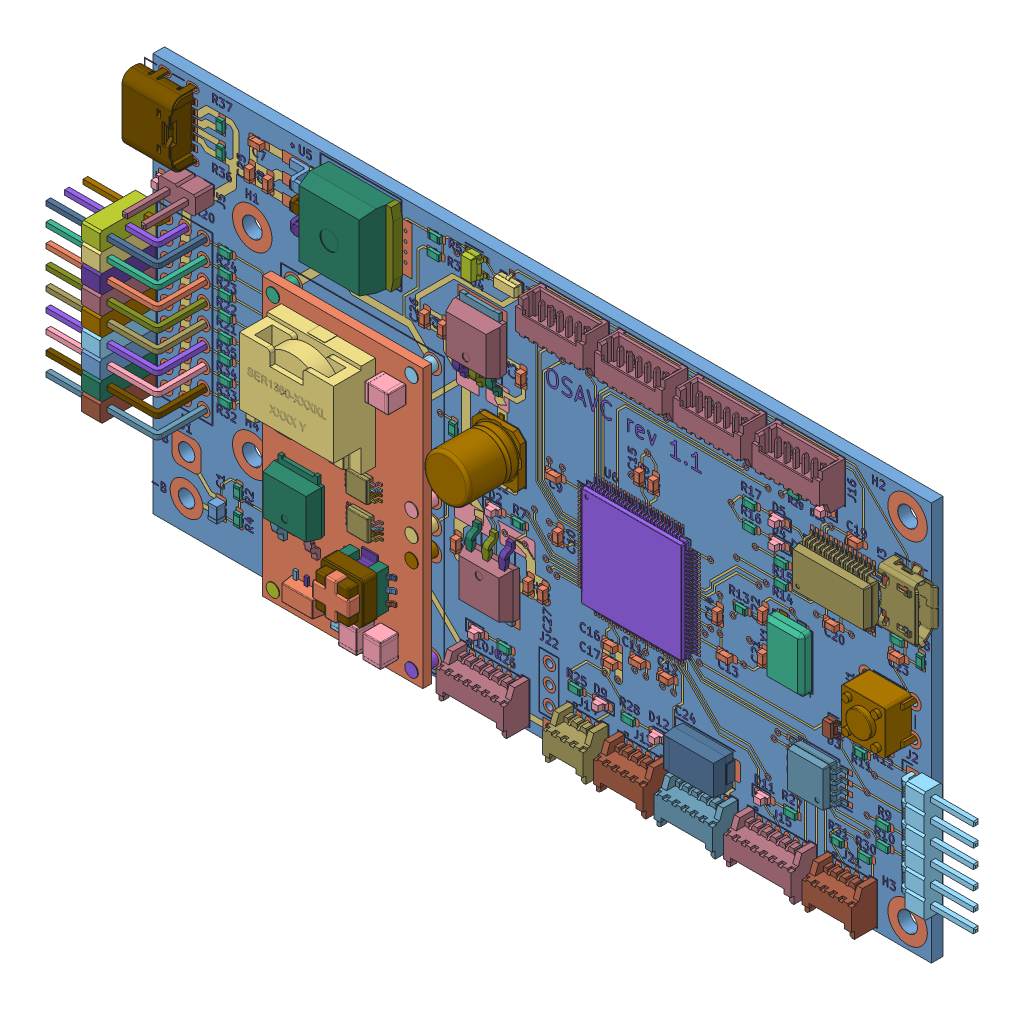
SolidWorks assembly OSAVC_rev1.1, configuration Default. Lengths in mm.
Overall size (122.32 54.61 12.06).
260 component instances, 123 part files, 0 mates.
Components (placement in the parent):
- OSAVC_rev1.1.step-1: OSAVC_rev1.1.step [Default] at origin size (122.32 54.61 12.06)
  - Local_CS_6c55.step-1: Local_CS_6c55.step [Default] at origin
  - Board_Geoms_6c55.step-1: Board_Geoms_6c55.step [Default] at origin size (107.79 54.61 2.3)
    - Pcb_6c55.step-1: Pcb_6c55.step [Default] at (-86.36 81.28 0) size (106.68 54.61 1.6)
    - PCB_Sketch_6c55.step-1: PCB_Sketch_6c55.step [Default] at origin
    - topPads_6c55_cut.step-1: topPads_6c55_cut.step [Default] at (0 0 0.02) size (105.36 53.51 0.01)
    - topTracks_6c55.step-1: topTracks_6c55.step [Default] at (-86.36 81.28 0.01) size (104.4 52.61 0.07)
    - topZones_6c55.step-1: topZones_6c55.step [Default] at (-86.36 81.28 0.01) size (10.98 18.86 0.02)
    - botPads_6c55.step-1: botPads_6c55.step [Default] at (-86.36 81.28 -1.62) size (105.31 53.51 0.01)
    - botTracks_6c55.step-1: botTracks_6c55.step [Default] at (-86.36 81.28 -1.61) size (93.18 51.32 0.63)
    - botSilks_69b0.step-1: botSilks_69b0.step [Default] at (-86.36 81.28 -1.67) size (102.66 52.04 0.03)
    - topSilks_6464.step-1: topSilks_6464.step [Default] at (-86.36 81.28 0.07) size (107.59 54.1 0.61)
  - Step_Models_6c55.step-1: Step_Models_6c55.step [Default] at origin size (122.32 53.45 12.06)
    - Top_6c55.step-1: Top_6c55.step [Default] at origin size (122.32 53.45 12.06)
      - C2_C_Elec_63x079_00006184c965.step-1: C2_C_Elec_63x079_00006184c965.step [Default] at (47.89 -22.72 0) x (0 -1 0) z (0 0 1) size (8.61 8.6 7.7)
        - C_Elec_63x77.step-1: C_Elec_63x77.step [Default] at origin size (8.61 8.6 7.7)
        - C_Elec_63x078.step-1: C_Elec_63x078.step [Default] at origin size (0.02 0.02 0.01)
      - J4_PinHeader_3x09_P2.54mm_Horizontal036_00006184cc7d.step-1: J4_PinHeader_3x09_P2.54mm_Horizontal036_00006184cc7d.step [Default] at (6.985 -38.735 0) x (-1 0 0) z (0 0 1) size (15.44 22.86 10.62)
        - PinHeader_3x09_P2.54mm_Horizontal.step-1: PinHeader_3x09_P2.54mm_Horizontal.step [Default] at origin size (2.54 2.54 7.62)
        - PinHeader_3x09_P2.54mm_Horizontal001.step-1: PinHeader_3x09_P2.54mm_Horizontal001.step [Default] at origin size (12.9 0.64 7.13)
        - PinHeader_3x09_P2.54mm_Horizontal002.step-1: PinHeader_3x09_P2.54mm_Horizontal002.step [Default] at origin size (10.36 0.64 4.59)
        - PinHeader_3x09_P2.54mm_Horizontal003.step-1: PinHeader_3x09_P2.54mm_Horizontal003.step [Default] at origin size (15.44 0.64 9.67)
        - PinHeader_3x09_P2.54mm_Horizontal004.step-1: PinHeader_3x09_P2.54mm_Horizontal004.step [Default] at origin size (2.54 2.54 7.62)
        - PinHeader_3x09_P2.54mm_Horizontal005.step-1: PinHeader_3x09_P2.54mm_Horizontal005.step [Default] at origin size (12.9 0.64 7.13)
        - PinHeader_3x09_P2.54mm_Horizontal006.step-1: PinHeader_3x09_P2.54mm_Horizontal006.step [Default] at origin size (10.36 0.64 4.59)
        - PinHeader_3x09_P2.54mm_Horizontal007.step-1: PinHeader_3x09_P2.54mm_Horizontal007.step [Default] at origin size (15.44 0.64 9.67)
        - PinHeader_3x09_P2.54mm_Horizontal008.step-1: PinHeader_3x09_P2.54mm_Horizontal008.step [Default] at origin size (2.54 2.54 7.62)
        - PinHeader_3x09_P2.54mm_Horizontal009.step-1: PinHeader_3x09_P2.54mm_Horizontal009.step [Default] at origin size (12.9 0.64 7.13)
        - PinHeader_3x09_P2.54mm_Horizontal010.step-1: PinHeader_3x09_P2.54mm_Horizontal010.step [Default] at origin size (10.36 0.64 4.59)
        - PinHeader_3x09_P2.54mm_Horizontal011.step-1: PinHeader_3x09_P2.54mm_Horizontal011.step [Default] at origin size (15.44 0.64 9.67)
        - PinHeader_3x09_P2.54mm_Horizontal012.step-1: PinHeader_3x09_P2.54mm_Horizontal012.step [Default] at origin size (2.54 2.54 7.62)
        - PinHeader_3x09_P2.54mm_Horizontal013.step-1: PinHeader_3x09_P2.54mm_Horizontal013.step [Default] at origin size (12.9 0.64 7.13)
        - PinHeader_3x09_P2.54mm_Horizontal014.step-1: PinHeader_3x09_P2.54mm_Horizontal014.step [Default] at origin size (10.36 0.64 4.59)
        - PinHeader_3x09_P2.54mm_Horizontal015.step-1: PinHeader_3x09_P2.54mm_Horizontal015.step [Default] at origin size (15.44 0.64 9.67)
        - PinHeader_3x09_P2.54mm_Horizontal016.step-1: PinHeader_3x09_P2.54mm_Horizontal016.step [Default] at origin size (2.54 2.54 7.62)
        - PinHeader_3x09_P2.54mm_Horizontal017.step-1: PinHeader_3x09_P2.54mm_Horizontal017.step [Default] at origin size (12.9 0.64 7.13)
        - PinHeader_3x09_P2.54mm_Horizontal018.step-1: PinHeader_3x09_P2.54mm_Horizontal018.step [Default] at origin size (10.36 0.64 4.59)
        - PinHeader_3x09_P2.54mm_Horizontal019.step-1: PinHeader_3x09_P2.54mm_Horizontal019.step [Default] at origin size (15.44 0.64 9.67)
        - PinHeader_3x09_P2.54mm_Horizontal020.step-1: PinHeader_3x09_P2.54mm_Horizontal020.step [Default] at origin size (2.54 2.54 7.62)
        - PinHeader_3x09_P2.54mm_Horizontal021.step-1: PinHeader_3x09_P2.54mm_Horizontal021.step [Default] at origin size (12.9 0.64 7.13)
        - PinHeader_3x09_P2.54mm_Horizontal022.step-1: PinHeader_3x09_P2.54mm_Horizontal022.step [Default] at origin size (10.36 0.64 4.59)
        - PinHeader_3x09_P2.54mm_Horizontal023.step-1: PinHeader_3x09_P2.54mm_Horizontal023.step [Default] at origin size (15.44 0.64 9.67)
        - PinHeader_3x09_P2.54mm_Horizontal024.step-1: PinHeader_3x09_P2.54mm_Horizontal024.step [Default] at origin size (2.54 2.54 7.62)
        - PinHeader_3x09_P2.54mm_Horizontal025.step-1: PinHeader_3x09_P2.54mm_Horizontal025.step [Default] at origin size (12.9 0.64 7.13)
        - PinHeader_3x09_P2.54mm_Horizontal026.step-1: PinHeader_3x09_P2.54mm_Horizontal026.step [Default] at origin size (10.36 0.64 4.59)
        - PinHeader_3x09_P2.54mm_Horizontal027.step-1: PinHeader_3x09_P2.54mm_Horizontal027.step [Default] at origin size (15.44 0.64 9.67)
        - PinHeader_3x09_P2.54mm_Horizontal028.step-1: PinHeader_3x09_P2.54mm_Horizontal028.step [Default] at origin size (2.54 2.54 7.62)
        - PinHeader_3x09_P2.54mm_Horizontal029.step-1: PinHeader_3x09_P2.54mm_Horizontal029.step [Default] at origin size (12.9 0.64 7.13)
        - PinHeader_3x09_P2.54mm_Horizontal030.step-1: PinHeader_3x09_P2.54mm_Horizontal030.step [Default] at origin size (10.36 0.64 4.59)
        - PinHeader_3x09_P2.54mm_Horizontal031.step-1: PinHeader_3x09_P2.54mm_Horizontal031.step [Default] at origin size (15.44 0.64 9.67)
        - PinHeader_3x09_P2.54mm_Horizontal032.step-1: PinHeader_3x09_P2.54mm_Horizontal032.step [Default] at origin size (2.54 2.54 7.62)
        - PinHeader_3x09_P2.54mm_Horizontal033.step-1: PinHeader_3x09_P2.54mm_Horizontal033.step [Default] at origin size (12.9 0.64 7.13)
        - PinHeader_3x09_P2.54mm_Horizontal034.step-1: PinHeader_3x09_P2.54mm_Horizontal034.step [Default] at origin size (10.36 0.64 4.59)
        - PinHeader_3x09_P2.54mm_Horizontal035.step-1: PinHeader_3x09_P2.54mm_Horizontal035.step [Default] at origin size (15.44 0.64 9.67)
      - J13_Picoblade_horizontal_4p_00006184cca8.step-1: J13_Picoblade_horizontal_4p_00006184cca8.step [Default] at (65.405 -49.53 0) x (1 0 0) z (0 -1 0) size (6.75 5.8 5.5)
        - 530480410.step-1: 530480410.step [Default] at (1.875 1.9 3.475) x (-1 0 0) z (0 1 0) size (6.75 5.5 5.8)
      - J14_Picoblade_horizontal_3p_00006184ccd2.step-1: J14_Picoblade_horizontal_3p_00006184ccd2.step [Default] at (58.42 -49.53 0) x (1 0 0) z (0 -1 0) size (5.5 5.8 5.5)
        - 530480310.step-1: 530480310.step [Default] at (1.25 1.9 3.475) x (-1 0 0) z (0 1 0) size (5.5 5.5 5.8)
      - J15_Picoblade_horizontal_6p_00006184ccff.step-1: J15_Picoblade_horizontal_6p_00006184ccff.step [Default] at (83.185 -49.53 0) x (1 0 0) z (0 -1 0) size (9.25 5.8 5.5)
        - 530480610.step-1: 530480610.step [Default] at (3.125 1.9 3.475) x (-1 0 0) z (0 1 0) size (9.25 5.5 5.8)
      - J15_Picoblade_horizontal_6p_00006184ccff.step-2: J15_Picoblade_horizontal_6p_00006184ccff.step [Default] at (93.345 -5.08 0) x (-1 0 0) z (0 1 0) size (9.25 5.8 5.5)
        - 530480610.step-1: 530480610.step [Default] at (3.125 1.9 3.475) x (-1 0 0) z (0 1 0) size (9.25 5.5 5.8)
      - J15_Picoblade_horizontal_6p_00006184ccff.step-3: J15_Picoblade_horizontal_6p_00006184ccff.step [Default] at (82.55 -5.08 0) x (-1 0 0) z (0 1 0) size (9.25 5.8 5.5)
        - 530480610.step-1: 530480610.step [Default] at (3.125 1.9 3.475) x (-1 0 0) z (0 1 0) size (9.25 5.5 5.8)
      - J15_Picoblade_horizontal_6p_00006184ccff.step-4: J15_Picoblade_horizontal_6p_00006184ccff.step [Default] at (71.755 -5.08 0) x (-1 0 0) z (0 1 0) size (9.25 5.8 5.5)
        - 530480610.step-1: 530480610.step [Default] at (3.125 1.9 3.475) x (-1 0 0) z (0 1 0) size (9.25 5.5 5.8)
      - J20_Picoblade_horizontal_5p_00006184cddf.step-1: J20_Picoblade_horizontal_5p_00006184cddf.step [Default] at (73.66 -49.53 0) x (1 0 0) z (0 -1 0) size (8 5.8 5.5)
        - 530480510.step-1: 530480510.step [Default] at (2.5 1.9 3.475) x (-1 0 0) z (0 1 0) size (8 5.5 5.8)
      - J13_Picoblade_horizontal_4p_00006184cca8.step-2: J13_Picoblade_horizontal_4p_00006184cca8.step [Default] at (93.98 -49.53 0) x (1 0 0) z (0 -1 0) size (6.75 5.8 5.5)
        - 530480410.step-1: 530480410.step [Default] at (1.875 1.9 3.475) x (-1 0 0) z (0 1 0) size (6.75 5.5 5.8)
      - U5_CQ assembly_00006184d1ab.step-1: U5_CQ assembly_00006184d1ab.step [Default] at (28.575 -5.715 0) size (15 10 4.42)
        - a52d3816-9c39-11ed-93f0-dde97e994e83.step-1: a52d3816-9c39-11ed-93f0-dde97e994e83.step [Default] at origin size (15 10 4.42)
          - a52d3817-9c39-11ed-93f0-dde97e994e83.step-1: a52d3817-9c39-11ed-93f0-dde97e994e83.step [Default] at origin size (9.25 10 4.4)
            - a52d3817-9c39-11ed-93f0-dde97e994e83_part.step-1: a52d3817-9c39-11ed-93f0-dde97e994e83_part.step [Default] at origin size (9.25 10 4.4)
          - a52d3818-9c39-11ed-93f0-dde97e994e83.step-1: a52d3818-9c39-11ed-93f0-dde97e994e83.step [Default] at origin size (7.55 10 1.27)
            - a52d3818-9c39-11ed-93f0-dde97e994e83_part.step-1: a52d3818-9c39-11ed-93f0-dde97e994e83_part.step [Default] at origin size (7.55 10 1.27)
          - a52d3819-9c39-11ed-93f0-dde97e994e83.step-1: a52d3819-9c39-11ed-93f0-dde97e994e83.step [Default] at origin size (4.95 6.32 2.95)
            - a52d3819-9c39-11ed-93f0-dde97e994e83_part003.step-1: a52d3819-9c39-11ed-93f0-dde97e994e83_part003.step [Default] at origin size (4.95 6.32 2.95)
              - a52d3819-9c39-11ed-93f0-dde97e994e83_part.step-1: a52d3819-9c39-11ed-93f0-dde97e994e83_part.step [Default] at origin size (4.95 1.24 2.95)
              - a52d3819-9c39-11ed-93f0-dde97e994e83_part001.step-1: a52d3819-9c39-11ed-93f0-dde97e994e83_part001.step [Default] at origin size (4.95 1.24 2.95)
              - a52d3819-9c39-11ed-93f0-dde97e994e83_part002.step-1: a52d3819-9c39-11ed-93f0-dde97e994e83_part002.step [Default] at origin size (4.95 1.24 2.95)
      - J15_Picoblade_horizontal_6p_00006184ccff.step-5: J15_Picoblade_horizontal_6p_00006184ccff.step [Default] at (43.815 -49.53 0) x (1 0 0) z (0 -1 0) size (9.25 5.8 5.5)
        - 530480610.step-1: 530480610.step [Default] at (3.125 1.9 3.475) x (-1 0 0) z (0 1 0) size (9.25 5.5 5.8)
      - U1_PTN78020W_EUK-7_00006189aa32.step-1: U1_PTN78020W_EUK-7_00006189aa32.step [Default] at (19.304 -52.578 0) x (1 0 0) z (0 -1 0) size (22 12 38)
        - Board^Voltage_regulator.STEP008.step-1: Board^Voltage_regulator.STEP008.step [Default] at origin size (22 6.34 38)
          - Board^Voltage_regulator.STEP.step-1: Board^Voltage_regulator.STEP.step [Default] at origin size (22 1.2 38)
          - Board^Voltage_regulator.STEP001.step-1: Board^Voltage_regulator.STEP001.step [Default] at origin size (1.75 6.34 1.75)
          - Board^Voltage_regulator.STEP002.step-1: Board^Voltage_regulator.STEP002.step [Default] at origin size (1.75 6.34 1.75)
          - Board^Voltage_regulator.STEP003.step-1: Board^Voltage_regulator.STEP003.step [Default] at origin size (1.75 6.34 1.75)
          - Board^Voltage_regulator.STEP004.step-1: Board^Voltage_regulator.STEP004.step [Default] at origin size (1.75 6.34 1.75)
          - Board^Voltage_regulator.STEP005.step-1: Board^Voltage_regulator.STEP005.step [Default] at origin size (1.75 6.34 1.75)
          - Board^Voltage_regulator.STEP006.step-1: Board^Voltage_regulator.STEP006.step [Default] at origin size (1.75 6.34 1.75)
          - Board^Voltage_regulator.STEP007.step-1: Board^Voltage_regulator.STEP007.step [Default] at origin size (1.75 6.34 1.75)
        - SMTCurrentSenseTransformer.STEP011.step-1: SMTCurrentSenseTransformer.STEP011.step [Default] at origin size (7.12 5.58 6.13)
          - SMTCurrentSenseTransformer.STEP.step-1: SMTCurrentSenseTransformer.STEP.step [Default] at (13.366 2.8 -8.2501) size (0.93 0.55 0.52)
          - SMTCurrentSenseTransformer.STEP001.step-1: SMTCurrentSenseTransformer.STEP001.step [Default] at (13.366 2.8 -8.2501) size (0.93 0.55 0.52)
          - SMTCurrentSenseTransformer.STEP002.step-1: SMTCurrentSenseTransformer.STEP002.step [Default] at (13.366 2.8 -8.2501) size (0.93 0.55 0.52)
          - SMTCurrentSenseTransformer.STEP003.step-1: SMTCurrentSenseTransformer.STEP003.step [Default] at (13.366 2.8 -8.2501) size (0.93 0.55 0.52)
          - SMTCurrentSenseTransformer.STEP004.step-1: SMTCurrentSenseTransformer.STEP004.step [Default] at (13.366 2.8 -8.2501) size (0.93 0.55 0.52)
          - SMTCurrentSenseTransformer.STEP005.step-1: SMTCurrentSenseTransformer.STEP005.step [Default] at (13.366 2.8 -8.2501) size (5.27 1.76 5.27)
          - SMTCurrentSenseTransformer.STEP006.step-1: SMTCurrentSenseTransformer.STEP006.step [Default] at (13.366 2.8 -8.2501) size (2.16 1.97 1.51)
          - SMTCurrentSenseTransformer.STEP007.step-1: SMTCurrentSenseTransformer.STEP007.step [Default] at (13.366 2.8 -8.2501) size (2.16 1.97 1.51)
          - SMTCurrentSenseTransformer.STEP008.step-1: SMTCurrentSenseTransformer.STEP008.step [Default] at (13.366 2.8 -8.2501) size (5.7 3.39 5.7)
          - SMTCurrentSenseTransformer.STEP009.step-1: SMTCurrentSenseTransformer.STEP009.step [Default] at (13.366 2.8 -8.2501) size (0.93 0.55 0.52)
          - SMTCurrentSenseTransformer.STEP010.step-1: SMTCurrentSenseTransformer.STEP010.step [Default] at (13.366 2.8 -8.2501) size (5.02 1.55 5.02)
        - MSOP-8.STEP010.step-1: MSOP-8.STEP010.step [Default] at origin size (4.9 1.1 3)
          - MSOP-8.STEP.step-1: MSOP-8.STEP.step [Default] at (12.6175 3.1325 -15.6358) x (0 -1 0) z (-1 0 0) size (0.67 0.44 1.43)
          - MSOP-8.STEP001.step-1: MSOP-8.STEP001.step [Default] at (12.6175 3.1325 -15.6358) x (0 -1 0) z (-1 0 0) size (0.67 0.44 1.43)
          - MSOP-8.STEP002.step-1: MSOP-8.STEP002.step [Default] at (12.6175 3.1325 -15.6358) x (0 -1 0) z (-1 0 0) size (0.67 0.44 1.43)
          - MSOP-8.STEP003.step-1: MSOP-8.STEP003.step [Default] at (12.6175 3.1325 -15.6358) x (0 -1 0) z (-1 0 0) size (0.67 0.44 1.43)
          - MSOP-8.STEP004.step-1: MSOP-8.STEP004.step [Default] at (12.6175 3.1325 -15.6358) x (0 -1 0) z (-1 0 0) size (0.67 0.44 1.43)
          - MSOP-8.STEP005.step-1: MSOP-8.STEP005.step [Default] at (12.6175 3.1325 -15.6358) x (0 -1 0) z (-1 0 0) size (0.15 2.39 1.73)
          - MSOP-8.STEP006.step-1: MSOP-8.STEP006.step [Default] at (12.6175 3.1325 -15.6358) x (0 -1 0) z (-1 0 0) size (0.67 0.44 1.43)
          - MSOP-8.STEP007.step-1: MSOP-8.STEP007.step [Default] at (12.6175 3.1325 -15.6358) x (0 -1 0) z (-1 0 0) size (0.67 0.44 1.43)
          - MSOP-8.STEP008.step-1: MSOP-8.STEP008.step [Default] at (12.6175 3.1325 -15.6358) x (0 -1 0) z (-1 0 0) size (0.67 0.44 1.43)
          - MSOP-8.STEP009.step-1: MSOP-8.STEP009.step [Default] at (12.6175 3.1325 -15.6358) x (0 -1 0) z (-1 0 0) size (0.94 3 3.01)
        - MSOP-8.STEP021.step-1: MSOP-8.STEP021.step [Default] at origin size (4.9 1.1 3)
          - MSOP-8.STEP.step-1: MSOP-8.STEP.step [Default] at (12.5011 3.1325 -20.1358) x (0 -1 0) z (-1 0 0) size (0.67 0.44 1.43)
          - MSOP-8.STEP001.step-1: MSOP-8.STEP001.step [Default] at (12.5011 3.1325 -20.1358) x (0 -1 0) z (-1 0 0) size (0.67 0.44 1.43)
          - MSOP-8.STEP002.step-1: MSOP-8.STEP002.step [Default] at (12.5011 3.1325 -20.1358) x (0 -1 0) z (-1 0 0) size (0.67 0.44 1.43)
          - MSOP-8.STEP003.step-1: MSOP-8.STEP003.step [Default] at (12.5011 3.1325 -20.1358) x (0 -1 0) z (-1 0 0) size (0.67 0.44 1.43)
          - MSOP-8.STEP004.step-1: MSOP-8.STEP004.step [Default] at (12.5011 3.1325 -20.1358) x (0 -1 0) z (-1 0 0) size (0.67 0.44 1.43)
          - MSOP-8.STEP005.step-1: MSOP-8.STEP005.step [Default] at (12.5011 3.1325 -20.1358) x (0 -1 0) z (-1 0 0) size (0.15 2.39 1.73)
          - MSOP-8.STEP006.step-1: MSOP-8.STEP006.step [Default] at (12.5011 3.1325 -20.1358) x (0 -1 0) z (-1 0 0) size (0.67 0.44 1.43)
          - MSOP-8.STEP007.step-1: MSOP-8.STEP007.step [Default] at (12.5011 3.1325 -20.1358) x (0 -1 0) z (-1 0 0) size (0.67 0.44 1.43)
          - MSOP-8.STEP008.step-1: MSOP-8.STEP008.step [Default] at (12.5011 3.1325 -20.1358) x (0 -1 0) z (-1 0 0) size (0.67 0.44 1.43)
          - MSOP-8.STEP009.step-1: MSOP-8.STEP009.step [Default] at (12.5011 3.1325 -20.1358) x (0 -1 0) z (-1 0 0) size (0.94 3 3.01)
        - DPAK.STEP004.step-1: DPAK.STEP004.step [Default] at origin size (6.5 2.3 9.95)
          - DPAK.STEP.step-1: DPAK.STEP.step [Default] at (3.8382 3.3 -12.8868) size (1 1.4 3.06)
          - DPAK.STEP001.step-1: DPAK.STEP001.step [Default] at (3.8382 3.3 -12.8868) size (1 1.4 3.06)
          - DPAK.STEP002.step-1: DPAK.STEP002.step [Default] at (3.8382 3.3 -12.8868) size (6.5 2.3 7.05)
          - DPAK.STEP003.step-1: DPAK.STEP003.step [Default] at (3.8382 3.3 -12.8868) size (0.9 0.5 0.8)
        - SOT89.STEP004.step-1: SOT89.STEP004.step [Default] at origin size (4.5 1.5 4.13)
          - SOT89.STEP.step-1: SOT89.STEP.step [Default] at (4.7525 3.13 -2) x (-1 0 0) z (0 0 1) size (1.6 0.33 4.13)
          - SOT89.STEP001.step-1: SOT89.STEP001.step [Default] at (4.7525 3.13 -2) x (-1 0 0) z (0 0 1) size (0.47 0.33 1.48)
          - SOT89.STEP002.step-1: SOT89.STEP002.step [Default] at (4.7525 3.13 -2) x (-1 0 0) z (0 0 1) size (0.47 0.33 1.48)
          - SOT89.STEP003.step-1: SOT89.STEP003.step [Default] at (4.7525 3.13 -2) x (-1 0 0) z (0 0 1) size (4.5 1.5 2.5)
        - Coilcraft-SER1360.STEP.step-1: Coilcraft-SER1360.STEP.step [Default] at (7.55 2.8 -28.05) x (0 0 1) z (-1 0 0) size (13 5.81 12.9)
        - SMD_Capacitor_1210_1210.STEP.step-1: SMD_Capacitor_1210_1210.STEP.step [Default] at (15.94 4.04 -1.9) x (0 0 1) z (-1 0 0) size (3.2 2.5 2.5)
        - SMD_Capacitor_1210_1210.STEP.step-2: SMD_Capacitor_1210_1210.STEP.step [Default] at (12.64 4.04 -1.9) x (0 0 1) z (-1 0 0) size (3.2 2.5 2.5)
        - SMD_Capacitor_1210_1210.STEP.step-3: SMD_Capacitor_1210_1210.STEP.step [Default] at (16.6 4.04 -32.26) size (3.2 2.5 2.5)
        - SMD_Capacitor_0805_0805.STEP.step-1: SMD_Capacitor_0805_0805.STEP.step [Default] at (9.715 3.44 -1.625) x (0 0 -1) z (-1 0 0) size (2 1.3 1.25)
      - J15_Picoblade_horizontal_6p_00006184ccff.step-6: J15_Picoblade_horizontal_6p_00006184ccff.step [Default] at (60.96 -5.08 0) x (-1 0 0) z (0 1 0) size (9.25 5.8 5.5)
        - 530480610.step-1: 530480610.step [Default] at (3.125 1.9 3.475) x (-1 0 0) z (0 1 0) size (9.25 5.5 5.8)
      - Y1_SMD_crystal005_0000618b2749.step-1: Y1_SMD_crystal005_0000618b2749.step [Default] at (87.757 -27.051 0) x (0 1 0) z (0 0 1) size (8.22 5.2 1.5)
        - SMD_crystal.step-1: SMD_crystal.step [Default] at origin size (7.5 5.2 1.4)
        - SMD_crystal001.step-1: SMD_crystal001.step [Default] at origin size (1.92 1.12 0.1)
        - SMD_crystal002.step-1: SMD_crystal002.step [Default] at origin size (1.92 1.12 0.1)
        - SMD_crystal003.step-1: SMD_crystal003.step [Default] at origin size (1.92 1.12 0.1)
        - SMD_crystal004.step-1: SMD_crystal004.step [Default] at origin size (1.92 1.12 0.1)
      - J3_10118193003_0000618b348a.step-1: J3_10118193003_0000618b348a.step [Default] at (104.805 -12.065 0) x (0 1 0) z (1 0 0) size (7.87 3.61 5.71)
        - 10118193002.step-1: 10118193002.step [Default] at origin size (7.87 3.61 5.71)
          - 10118193.step-1: 10118193.step [Default] at (-0.19 0.055 -0.3676) size (6.89 2.35 4.32)
          - 10118193001.step-1: 10118193001.step [Default] at (-0.19 0.055 -0.3676) size (7.87 3.61 5.67)
      - U3_CQ assembly_0000618ecb8d.step-1: U3_CQ assembly_0000618ecb8d.step [Default] at (46.99 -38.8526 0) x (0 -1 0) z (0 0 1) size (9.9 6.5 2.32)
        - 98f8d7e0-9c39-11ed-93f0-dde97e994e83.step-1: 98f8d7e0-9c39-11ed-93f0-dde97e994e83.step [Default] at origin size (9.9 6.5 2.32)
          - 98f8d7e1-9c39-11ed-93f0-dde97e994e83.step-1: 98f8d7e1-9c39-11ed-93f0-dde97e994e83.step [Default] at origin size (6.22 6.5 2.3)
            - 98f8d7e1-9c39-11ed-93f0-dde97e994e83_part.step-1: 98f8d7e1-9c39-11ed-93f0-dde97e994e83_part.step [Default] at origin size (6.22 6.5 2.3)
          - 98f8d7e2-9c39-11ed-93f0-dde97e994e83.step-1: 98f8d7e2-9c39-11ed-93f0-dde97e994e83.step [Default] at origin size (5.24 5.4 0.5)
            - 98f8d7e2-9c39-11ed-93f0-dde97e994e83_part.step-1: 98f8d7e2-9c39-11ed-93f0-dde97e994e83_part.step [Default] at origin size (5.24 5.4 0.5)
          - 98f8d7e3-9c39-11ed-93f0-dde97e994e83.step-1: 98f8d7e3-9c39-11ed-93f0-dde97e994e83.step [Default] at origin size (3.55 5.55 1.44)
            - 98f8d7e3-9c39-11ed-93f0-dde97e994e83_part003.step-1: 98f8d7e3-9c39-11ed-93f0-dde97e994e83_part003.step [Default] at origin size (3.55 5.55 1.44)
              - 98f8d7e3-9c39-11ed-93f0-dde97e994e83_part.step-1: 98f8d7e3-9c39-11ed-93f0-dde97e994e83_part.step [Default] at origin size (3.55 0.99 1.44)
              - 98f8d7e3-9c39-11ed-93f0-dde97e994e83_part001.step-1: 98f8d7e3-9c39-11ed-93f0-dde97e994e83_part001.step [Default] at origin size (3.55 0.99 1.44)
              - 98f8d7e3-9c39-11ed-93f0-dde97e994e83_part002.step-1: 98f8d7e3-9c39-11ed-93f0-dde97e994e83_part002.step [Default] at origin size (3.55 0.99 1.44)
      - U3_CQ assembly_0000618ecb8d.step-2: U3_CQ assembly_0000618ecb8d.step [Default] at (45.212 -10.8044 0) x (0 1 0) z (0 0 1) size (9.9 6.5 2.32)
        - 98f8d7e0-9c39-11ed-93f0-dde97e994e83.step-1: 98f8d7e0-9c39-11ed-93f0-dde97e994e83.step [Default] at origin size (9.9 6.5 2.32)
          - 98f8d7e1-9c39-11ed-93f0-dde97e994e83.step-1: 98f8d7e1-9c39-11ed-93f0-dde97e994e83.step [Default] at origin size (6.22 6.5 2.3)
            - 98f8d7e1-9c39-11ed-93f0-dde97e994e83_part.step-1: 98f8d7e1-9c39-11ed-93f0-dde97e994e83_part.step [Default] at origin size (6.22 6.5 2.3)
          - 98f8d7e2-9c39-11ed-93f0-dde97e994e83.step-1: 98f8d7e2-9c39-11ed-93f0-dde97e994e83.step [Default] at origin size (5.24 5.4 0.5)
            - 98f8d7e2-9c39-11ed-93f0-dde97e994e83_part.step-1: 98f8d7e2-9c39-11ed-93f0-dde97e994e83_part.step [Default] at origin size (5.24 5.4 0.5)
          - 98f8d7e3-9c39-11ed-93f0-dde97e994e83.step-1: 98f8d7e3-9c39-11ed-93f0-dde97e994e83.step [Default] at origin size (3.55 5.55 1.44)
            - 98f8d7e3-9c39-11ed-93f0-dde97e994e83_part003.step-1: 98f8d7e3-9c39-11ed-93f0-dde97e994e83_part003.step [Default] at origin size (3.55 5.55 1.44)
              - 98f8d7e3-9c39-11ed-93f0-dde97e994e83_part.step-1: 98f8d7e3-9c39-11ed-93f0-dde97e994e83_part.step [Default] at origin size (3.55 0.99 1.44)
              - 98f8d7e3-9c39-11ed-93f0-dde97e994e83_part001.step-1: 98f8d7e3-9c39-11ed-93f0-dde97e994e83_part001.step [Default] at origin size (3.55 0.99 1.44)
              - 98f8d7e3-9c39-11ed-93f0-dde97e994e83_part002.step-1: 98f8d7e3-9c39-11ed-93f0-dde97e994e83_part002.step [Default] at origin size (3.55 0.99 1.44)
      - J23_USB4125-GF-A_000061969e33.step-1: J23_USB4125-GF-A_000061969e33.step [Default] at (-0.96 -5.58 0) x (0 -1 0) z (-1 0 0) size (8.95 4.43 7.12)
        - USB4125-GF-A_PART1.step-1: USB4125-GF-A_PART1.step [Default] at origin size (8.95 4.43 7.12)
      - C1_C_0805_2012Metric_00006184c954.step-1: C1_C_0805_2012Metric_00006184c954.step [Default] at (9.39 -49.22 0) x (0 -1 0) z (0 0 1) size (2 1.25 1.25)
      - C3_C_0603_1608Metric_00006184c976.step-1: C3_C_0603_1608Metric_00006184c976.step [Default] at (50.8 -12.954 0) x (0 1 0) z (0 0 1) size (1.6 0.8 0.8)
      - C3_C_0603_1608Metric_00006184c976.step-2: C3_C_0603_1608Metric_00006184c976.step [Default] at (40.14 -12.47 0) x (0 1 0) z (0 0 1) size (1.6 0.8 0.8)
      - C3_C_0603_1608Metric_00006184c976.step-3: C3_C_0603_1608Metric_00006184c976.step [Default] at (41.91 -37.084 0) x (0 -1 0) z (0 0 1) size (1.6 0.8 0.8)
      - C3_C_0603_1608Metric_00006184c976.step-4: C3_C_0603_1608Metric_00006184c976.step [Default] at (51.816 -37.084 0) x (0 -1 0) z (0 0 1) size (1.6 0.8 0.8)
      - C3_C_0603_1608Metric_00006184c976.step-5: C3_C_0603_1608Metric_00006184c976.step [Default] at (14.605 -3.175 0) x (-1 0 0) z (0 0 1) size (1.6 0.8 0.8)
      - C3_C_0603_1608Metric_00006184c976.step-6: C3_C_0603_1608Metric_00006184c976.step [Default] at (16.14 -7.22 0) x (0 1 0) z (0 0 1) size (1.6 0.8 0.8)
      - C3_C_0603_1608Metric_00006184c976.step-7: C3_C_0603_1608Metric_00006184c976.step [Default] at (55.88 -29.21 0) x (0 1 0) z (0 0 1) size (1.6 0.8 0.8)
      - C3_C_0603_1608Metric_00006184c976.step-8: C3_C_0603_1608Metric_00006184c976.step [Default] at (70.612 -38.608 0) x (-1 0 0) z (0 0 1) size (1.6 0.8 0.8)
      - C3_C_0603_1608Metric_00006184c976.step-9: C3_C_0603_1608Metric_00006184c976.step [Default] at (67.056 -16.51 0) x (0 1 0) z (0 0 1) size (1.6 0.8 0.8)
      - C3_C_0603_1608Metric_00006184c976.step-10: C3_C_0603_1608Metric_00006184c976.step [Default] at (62.992 -38.608 0) size (1.6 0.8 0.8)
      - C3_C_0603_1608Metric_00006184c976.step-11: C3_C_0603_1608Metric_00006184c976.step [Default] at (62.992 -40.64 0) size (1.6 0.8 0.8)
      - C3_C_0603_1608Metric_00006184c976.step-12: C3_C_0603_1608Metric_00006184c976.step [Default] at (13.64 -7.22 0) x (0 1 0) z (0 0 1) size (1.6 0.8 0.8)
      - C3_C_0603_1608Metric_00006184c976.step-13: C3_C_0603_1608Metric_00006184c976.step [Default] at (37.592 -12.446 0) x (0 1 0) z (0 0 1) size (1.6 0.8 0.8)
      - C3_C_0603_1608Metric_00006184c976.step-14: C3_C_0603_1608Metric_00006184c976.step [Default] at (53.848 -37.084 0) x (0 -1 0) z (0 0 1) size (1.6 0.8 0.8)
      - D6_SOT_23_00006184cb73.step-1: D6_SOT_23_00006184cb73.step [Default] at (14.605 -34.29 0) size (2.5 3 1.2)
      - D6_SOT_23_00006184cb73.step-2: D6_SOT_23_00006184cb73.step [Default] at (14.605 -29.845 0) size (2.5 3 1.2)
      - D8_LED_0603_1608Metric_00006184cb9b.step-1: D8_LED_0603_1608Metric_00006184cb9b.step [Default] at (1.27 -14.478 0) x (0 1 0) z (0 0 1) size (1.6 0.8 1.1)
      - D8_LED_0603_1608Metric_00006184cb9b.step-2: D8_LED_0603_1608Metric_00006184cb9b.step [Default] at (61.64 -46.22 0) x (-1 0 0) z (0 0 1) size (1.6 0.8 1.1)
      - D8_LED_0603_1608Metric_00006184cb9b.step-3: D8_LED_0603_1608Metric_00006184cb9b.step [Default] at (44.64 -46.22 0) size (1.6 0.8 1.1)
      - D8_LED_0603_1608Metric_00006184cb9b.step-4: D8_LED_0603_1608Metric_00006184cb9b.step [Default] at (83.89 -46.22 0) size (1.6 0.8 1.1)
      - D8_LED_0603_1608Metric_00006184cb9b.step-5: D8_LED_0603_1608Metric_00006184cb9b.step [Default] at (69.39 -46.22 0) x (-1 0 0) z (0 0 1) size (1.6 0.8 1.1)
      - D8_LED_0603_1608Metric_00006184cb9b.step-6: D8_LED_0603_1608Metric_00006184cb9b.step [Default] at (92.14 -7.97 0) x (-1 0 0) z (0 0 1) size (1.6 0.8 1.1)
      - J2_PinHeader_1x06_P254mm_Horizontal_00006184cc31.step-1: J2_PinHeader_1x06_P254mm_Horizontal_00006184cc31.step [Default] at (104.14 -33.655 0) size (10.36 15.24 5.54)
      - D6_SOT_23_00006184cb73.step-3: D6_SOT_23_00006184cb73.step [Default] at (49.276 -2.54 0) x (0 1 0) z (0 0 1) size (2.5 3 1.2)
      - R3_R_0603_1608Metric_00006184ceac.step-1: R3_R_0603_1608Metric_00006184ceac.step [Default] at (38.81 -4.318 0) size (1.6 0.8 0.45)
      - R3_R_0603_1608Metric_00006184ceac.step-2: R3_R_0603_1608Metric_00006184ceac.step [Default] at (100.33 -41.275 0) x (-1 0 0) z (0 0 1) size (1.6 0.8 0.45)
      - R3_R_0603_1608Metric_00006184ceac.step-3: R3_R_0603_1608Metric_00006184ceac.step [Default] at (100.33 -43.815 0) x (-1 0 0) z (0 0 1) size (1.6 0.8 0.45)
      - R3_R_0603_1608Metric_00006184ceac.step-4: R3_R_0603_1608Metric_00006184ceac.step [Default] at (97.155 -34.29 0) x (-1 0 0) z (0 0 1) size (1.6 0.8 0.45)
      - R3_R_0603_1608Metric_00006184ceac.step-5: R3_R_0603_1608Metric_00006184ceac.step [Default] at (100.33 -32.385 0) size (1.6 0.8 0.45)
      - R3_R_0603_1608Metric_00006184ceac.step-6: R3_R_0603_1608Metric_00006184ceac.step [Default] at (80.772 -25.4 0) size (1.6 0.8 0.45)
      - R3_R_0603_1608Metric_00006184ceac.step-7: R3_R_0603_1608Metric_00006184ceac.step [Default] at (86.36 -19.685 0) x (-1 0 0) z (0 0 1) size (1.6 0.8 0.45)
      - R3_R_0603_1608Metric_00006184ceac.step-8: R3_R_0603_1608Metric_00006184ceac.step [Default] at (86.36 -17.145 0) x (-1 0 0) z (0 0 1) size (1.6 0.8 0.45)
      - R3_R_0603_1608Metric_00006184ceac.step-9: R3_R_0603_1608Metric_00006184ceac.step [Default] at (3.81 -15.494 0) x (-1 0 0) z (0 0 1) size (1.6 0.8 0.45)
      - R3_R_0603_1608Metric_00006184ceac.step-10: R3_R_0603_1608Metric_00006184ceac.step [Default] at (10.16 -26.035 0) size (1.6 0.8 0.45)
      - R3_R_0603_1608Metric_00006184ceac.step-11: R3_R_0603_1608Metric_00006184ceac.step [Default] at (10.16 -23.495 0) size (1.6 0.8 0.45)
      - R3_R_0603_1608Metric_00006184ceac.step-12: R3_R_0603_1608Metric_00006184ceac.step [Default] at (10.16 -20.955 0) size (1.6 0.8 0.45)
      - R3_R_0603_1608Metric_00006184ceac.step-13: R3_R_0603_1608Metric_00006184ceac.step [Default] at (10.16 -18.415 0) size (1.6 0.8 0.45)
      - R3_R_0603_1608Metric_00006184ceac.step-14: R3_R_0603_1608Metric_00006184ceac.step [Default] at (58.14 -46.22 0) size (1.6 0.8 0.45)
      - R3_R_0603_1608Metric_00006184ceac.step-15: R3_R_0603_1608Metric_00006184ceac.step [Default] at (48.39 -46.22 0) x (-1 0 0) z (0 0 1) size (1.6 0.8 0.45)
      - R3_R_0603_1608Metric_00006184ceac.step-16: R3_R_0603_1608Metric_00006184ceac.step [Default] at (65.39 -46.22 0) size (1.6 0.8 0.45)
      - R3_R_0603_1608Metric_00006184ceac.step-17: R3_R_0603_1608Metric_00006184ceac.step [Default] at (88.14 -7.97 0) size (1.6 0.8 0.45)
      - R3_R_0603_1608Metric_00006184ceac.step-18: R3_R_0603_1608Metric_00006184ceac.step [Default] at (97.79 -46.355 0) x (-1 0 0) z (0 0 1) size (1.6 0.8 0.45)
      - R3_R_0603_1608Metric_00006184ceac.step-19: R3_R_0603_1608Metric_00006184ceac.step [Default] at (93.98 -46.355 0) x (-1 0 0) z (0 0 1) size (1.6 0.8 0.45)
      - R3_R_0603_1608Metric_00006184ceac.step-20: R3_R_0603_1608Metric_00006184ceac.step [Default] at (10.16 -36.195 0) x (-1 0 0) z (0 0 1) size (1.6 0.8 0.45)
      - R3_R_0603_1608Metric_00006184ceac.step-21: R3_R_0603_1608Metric_00006184ceac.step [Default] at (10.16 -31.115 0) x (-1 0 0) z (0 0 1) size (1.6 0.8 0.45)
      - R3_R_0603_1608Metric_00006184ceac.step-22: R3_R_0603_1608Metric_00006184ceac.step [Default] at (10.16 -28.575 0) x (-1 0 0) z (0 0 1) size (1.6 0.8 0.45)
      - U4_SOT_23_5_00006184d16f.step-1: U4_SOT_23_5_00006184d16f.step [Default] at (44.45 -2.54 0) size (2.8 2.9 1.55)
      - U6_TQFP_100_14x14mm_P05mm_00006184d23a.step-1: U6_TQFP_100_14x14mm_P05mm_00006184d23a.step [Default] at (66.675 -27.94 0) size (16 16 1.1)
      - SW1_SW_PUSH_6mm_h4.3mm_000061854ea1.step-1: SW1_SW_PUSH_6mm_h4.3mm_000061854ea1.step [Default] at (97.79 -24.765 0) size (7.17 6 7.8)
      - C3_C_0603_1608Metric_00006184c976.step-15: C3_C_0603_1608Metric_00006184c976.step [Default] at (55.245 -22.352 0) x (-1 0 0) z (0 0 1) size (1.6 0.8 0.8)
      - C3_C_0603_1608Metric_00006184c976.step-16: C3_C_0603_1608Metric_00006184c976.step [Default] at (78.74 -32.004 0) size (1.6 0.8 0.8)
      - C3_C_0603_1608Metric_00006184c976.step-17: C3_C_0603_1608Metric_00006184c976.step [Default] at (68.961 -16.51 0) x (0 1 0) z (0 0 1) size (1.6 0.8 0.8)
      - C24_CP_EIA_7343_30_AVX_N_00006185f6b5.step-1: C24_CP_EIA_7343_30_AVX_N_00006185f6b5.step [Default] at (76.2 -45.085 0) size (7.3 4.3 2.8)
      - R3_R_0603_1608Metric_00006184ceac.step-23: R3_R_0603_1608Metric_00006184ceac.step [Default] at (41.39 -23.72 0) x (0 1 0) z (0 0 1) size (1.6 0.8 0.45)
      - C3_C_0603_1608Metric_00006184c976.step-18: C3_C_0603_1608Metric_00006184c976.step [Default] at (96.52 -9.525 0) x (-1 0 0) z (0 0 1) size (1.6 0.8 0.8)
      - R3_R_0603_1608Metric_00006184ceac.step-24: R3_R_0603_1608Metric_00006184ceac.step [Default] at (82.042 -15.113 0) size (1.6 0.8 0.45)
      - R3_R_0603_1608Metric_00006184ceac.step-25: R3_R_0603_1608Metric_00006184ceac.step [Default] at (102.235 -18.415 0) x (-1 0 0) z (0 0 1) size (1.6 0.8 0.45)
      - R3_R_0603_1608Metric_00006184ceac.step-26: R3_R_0603_1608Metric_00006184ceac.step [Default] at (105.41 -19.304 0) x (0 -1 0) z (0 0 1) size (1.6 0.8 0.45)
      - R3_R_0603_1608Metric_00006184ceac.step-27: R3_R_0603_1608Metric_00006184ceac.step [Default] at (82.042 -12.319 0) size (1.6 0.8 0.45)
      - D8_LED_0603_1608Metric_00006184cb9b.step-7: D8_LED_0603_1608Metric_00006184cb9b.step [Default] at (85.852 -15.113 0) x (-1 0 0) z (0 0 1) size (1.6 0.8 1.1)
      - D8_LED_0603_1608Metric_00006184cb9b.step-8: D8_LED_0603_1608Metric_00006184cb9b.step [Default] at (85.852 -12.319 0) x (-1 0 0) z (0 0 1) size (1.6 0.8 1.1)
      - D3_SOT_323_SC_70_000061899956.step-1: D3_SOT_323_SC_70_000061899956.step [Default] at (93.345 -33.02 0) x (-1 0 0) z (0 0 1) size (2 2 1.05)
      - C3_C_0603_1608Metric_00006184c976.step-19: C3_C_0603_1608Metric_00006184c976.step [Default] at (93.345 -20.955 0) size (1.6 0.8 0.8)
      - U7_SSOP_28_53x102mm_P065mm_0000618a0f45.step-1: U7_SSOP_28_53x102mm_P065mm_0000618a0f45.step [Default] at (94.615 -15.24 0) x (0 1 0) z (0 0 1) size (7.8 10.2 2.1)
      - C3_C_0603_1608Metric_00006184c976.step-20: C3_C_0603_1608Metric_00006184c976.step [Default] at (102.235 -20.32 0) x (-1 0 0) z (0 0 1) size (1.6 0.8 0.8)
      - C3_C_0603_1608Metric_00006184c976.step-21: C3_C_0603_1608Metric_00006184c976.step [Default] at (83.947 -24.511 0) x (0 1 0) z (0 0 1) size (1.6 0.8 0.8)
      - C3_C_0603_1608Metric_00006184c976.step-22: C3_C_0603_1608Metric_00006184c976.step [Default] at (83.947 -29.591 0) x (0 -1 0) z (0 0 1) size (1.6 0.8 0.8)
      - C3_C_0603_1608Metric_00006184c976.step-23: C3_C_0603_1608Metric_00006184c976.step [Default] at (77.724 -27.686 0) x (0 1 0) z (0 0 1) size (1.6 0.8 0.8)
      - R3_R_0603_1608Metric_00006184ceac.step-28: R3_R_0603_1608Metric_00006184ceac.step [Default] at (97.155 -32.385 0) size (1.6 0.8 0.45)
      - C3_C_0603_1608Metric_00006184c976.step-24: C3_C_0603_1608Metric_00006184c976.step [Default] at (66.802 -38.608 0) x (-1 0 0) z (0 0 1) size (1.6 0.8 0.8)
      - R3_R_0603_1608Metric_00006184ceac.step-29: R3_R_0603_1608Metric_00006184ceac.step [Default] at (11.89 -45.97 0) x (0 -1 0) z (0 0 1) size (1.6 0.8 0.45)
      - R3_R_0603_1608Metric_00006184ceac.step-30: R3_R_0603_1608Metric_00006184ceac.step [Default] at (11.89 -49.22 0) x (0 -1 0) z (0 0 1) size (1.6 0.8 0.45)
      - J5_PinHeader_1x02_P254mm_Vertical_0000618bbe19.step-1: J5_PinHeader_1x02_P254mm_Vertical_0000618bbe19.step [Default] at (7.112 -12.7 0) x (0 -1 0) z (0 0 1) size (2.54 5.08 11.54)
      - R3_R_0603_1608Metric_00006184ceac.step-31: R3_R_0603_1608Metric_00006184ceac.step [Default] at (38.91 -2.198 0) x (-1 0 0) z (0 0 1) size (1.6 0.8 0.45)
      - R3_R_0603_1608Metric_00006184ceac.step-32: R3_R_0603_1608Metric_00006184ceac.step [Default] at (50.292 -30.48 0) x (-1 0 0) z (0 0 1) size (1.6 0.8 0.45)
      - D8_LED_0603_1608Metric_00006184cb9b.step-9: D8_LED_0603_1608Metric_00006184cb9b.step [Default] at (46.99 -30.48 0) size (1.6 0.8 1.1)
      - R3_R_0603_1608Metric_00006184ceac.step-33: R3_R_0603_1608Metric_00006184ceac.step [Default] at (9.525 -6.85 0) x (0 -1 0) z (0 0 1) size (1.6 0.8 0.45)
      - R3_R_0603_1608Metric_00006184ceac.step-34: R3_R_0603_1608Metric_00006184ceac.step [Default] at (9.525 -3.675 0) x (0 1 0) z (0 0 1) size (1.6 0.8 0.45)
      - R3_R_0603_1608Metric_00006184ceac.step-35: R3_R_0603_1608Metric_00006184ceac.step [Default] at (10.16 -33.655 0) x (-1 0 0) z (0 0 1) size (1.6 0.8 0.45)
      - U9_SOIJ_8_53x53mm_P127mm_000061dd964d.step-1: U9_SOIJ_8_53x53mm_P127mm_000061dd964d.step [Default] at (91.39 -39.47 0) x (-1 0 0) z (0 0 1) size (7.94 5.3 2.01)
      - R3_R_0603_1608Metric_00006184ceac.step-36: R3_R_0603_1608Metric_00006184ceac.step [Default] at (87.64 -46.22 0) x (-1 0 0) z (0 0 1) size (1.6 0.8 0.45)
